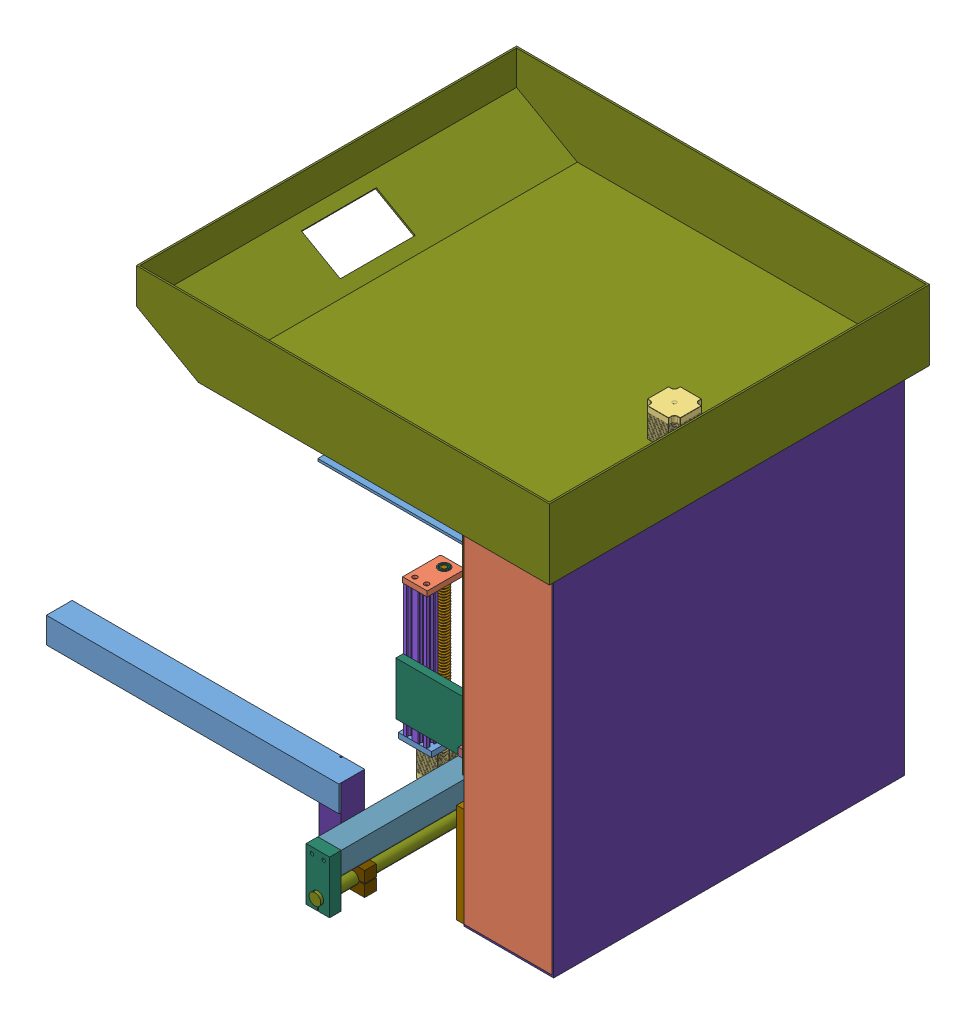
SolidWorks assembly Nueva Serigrafica, configuration Predeterminado. Lengths in mm.
Overall size (737.92 824.7 832.82).
71 component instances, 36 part files, 143 mates.
Components (placement in the parent):
- BASE DERECHA ACTUADOR LINEAL-1: BASE DERECHA ACTUADOR LINEAL [Predeterminado] at (30.0921 122.6863 -239.9315) x (0 1 0) z (0 0 -1) size (57 80 9)
- BASE LATERAL ACTUADOR LINEAL-1: BASE LATERAL ACTUADOR LINEAL [Predeterminado] at (22.5921 122.6863 182.0685) x (0 -1 0) z (0 0 1) size (42 65 9)
- SR Nema23 stepper motor with handwheel-1: SR Nema23 stepper motor with handwheel [Default] at (131.5379 118.3863 -326.6783) size (56.4 56.4 85)
- SOPORTE RODAMIENTO LATERAL-1: SOPORTE RODAMIENTO LATERAL [Predeterminado] at (32.5921 121.6863 -196.9315) x (0 1 0) z (0 0 -1) size (40 45 21)
- CARRO ACTUADOR LINEAL-1: CARRO ACTUADOR LINEAL [Predeterminado] at (40.0921 122.6863 164.8931) x (1 0 0) z (0 1 0) size (40 62 48)
- instrument ball bearing_68_am-1: instrument ball bearing_68_am [AFBMA 12.1.4.1 - 0080-19 - 10,DE,AC,10_68] at (40.0921 122.6863 188.0685) x (0 0 -1) z (1 0 0) size (6 19 19)
- instrument ball bearing_68_am-2: instrument ball bearing_68_am [AFBMA 12.1.4.1 - 0080-19 - 10,DE,AC,10_68] at (40.0921 122.6863 -199.9315) x (0 0 1) z (-1 0 0) size (6 19 19)
- VSlotRail_20X40X450-1: VSlotRail_20X40X450 [250mm] at (0.0921 132.6863 -239.9315) size (20 40 422)
- TORNILLO SINFINx400-1: TORNILLO SINFINx400 [Predeterminado] at (40.0921 122.6863 -77.9315) x (0 0 1) z (-1 0 0) size (289 16 16)
- SOPORTE ALUMINIO ACTUADOR SUPERIOR-1: SOPORTE ALUMINIO ACTUADOR SUPERIOR [Predeterminado] at (-22.6079 133.6863 -48.9315) x (0 0 -1) z (1 0 0) size (600 170 12.7)
- BARRA ACERO 20MM-1: BARRA ACERO 20MM [Predeterminado] at (30.0921 188.6863 -278.9315) x (0 0 1) z (-1 0 0) size (500 20 20)
- SOPORTE BARRA ACERO SUPERIOR-1: SOPORTE BARRA ACERO SUPERIOR [Predeterminado] at (30.0921 188.6863 206.3685) x (0 -1 0) z (0 0 1) size (40 55 12.7)
- SOPORTE BARRA ACERO SUPERIOR-2: SOPORTE BARRA ACERO SUPERIOR [Predeterminado] at (30.0921 188.6863 -281.2623) x (0 -1 0) z (0 0 1) size (40 55 12.7)
- CORREDERA SUPERIOR-1: CORREDERA SUPERIOR [Predeterminado] at (30.0921 188.6863 173.8931) x (0 -1 0) z (1 0 0) size (60 80 60)
- ANGULO 120X15X15X0.5In-1: ANGULO 120X15X15X0.5In [Predeterminado] at (72.7921 248.6863 133.8931) x (0 0 -1) z (0 1 0) size (120 150 150)
- RIEL SOPORTE-1: RIEL SOPORTE [Predeterminado] at (-57.2079 215.9863 133.8931) x (0 0 -1) z (-1 0 0) size (600 40 40)
- SOPORTE BARRA FRAME-1: SOPORTE BARRA FRAME [Predeterminado] at (-57.2079 190.9863 433.8931) x (-1 0 0) z (0 0 1) size (40 90 20)
- SOPORTE BARRA FRAME-2: SOPORTE BARRA FRAME [Predeterminado] at (-57.2079 190.9863 -186.1069) x (-1 0 0) z (0 0 1) size (40 90 20)
- BARRA ACERO 20MMX650-1: BARRA ACERO 20MMX650 [Predeterminado] at (-57.2079 165.9863 133.8931) x (1 0 0) z (0 1 0) size (20 650 20)
- RIEL 150mm-1: RIEL 150mm [Predeterminado] at (-97.2079 220.9863 373.8931) x (0 1 0) z (0 0 1) size (150 40 40)
- SOPORTE ACCESORIO-1: SOPORTE ACCESORIO [Predeterminado] at (-82.2079 165.9863 373.8931) x (0 -1 0) z (0 0 1) size (40 40 20)
- L ALUM 500X40X4mm-1: L ALUM 500X40X4mm [Predeterminado] at (-327.2079 291.9863 393.8931) x (0 -1 0) z (1 0 0) size (44 44 500)
- L ALUM 500X40X4mm-2: L ALUM 500X40X4mm [Predeterminado] at (-327.2079 291.9863 -106.1069) x (0 0 1) z (1 0 0) size (44 44 500)
- RIEL 150mm-2: RIEL 150mm [Predeterminado] at (-97.2079 220.9863 -86.1069) x (0 1 0) z (0 0 1) size (150 40 40)
- SOPORTE ACCESORIO-2: SOPORTE ACCESORIO [Predeterminado] at (-82.2079 165.9863 -106.1069) x (0 -1 0) z (0 0 1) size (40 40 20)
- SOPORTE LATERAL ALUMINIO SUPERIOR-1: SOPORTE LATERAL ALUMINIO SUPERIOR [Predeterminado] at (65.0921 348.6863 238.3685) x (0 -1 0) z (0 0 1) size (600 150 12.7)
- SOPORTE LATERAL ALUMINIO SUPERIOR-2: SOPORTE LATERAL ALUMINIO SUPERIOR [Predeterminado] at (65.0921 348.6863 -348.9315) x (0 -1 0) z (0 0 1) size (600 150 12.7)
- SOPORTE STEPPER DE REGISTRO-1: SOPORTE STEPPER DE REGISTRO [Predeterminado] at (-69.2332 426.7015 -48.9315) x (0 0 1) z (0.999998 -0.002087 0) size (60 80 12.7)
- SR Nema23 stepper motor with handwheel-2: SR Nema23 stepper motor with handwheel [Default] at (21.2027 421.3828 -140.9472) x (0 0 -1) z (-0.999998 0.002087 0) size (56.4 56.4 85)
- SOPORTE RODAMIENTO LATERAL-2: SOPORTE RODAMIENTO LATERAL [Predeterminado] at (-104.2383 424.2745 -47.9315) x (0 0 -1) z (-0.999998 0.002087 0) size (40 45 21)
- UNION STEPPER GUIA-1: UNION STEPPER GUIA [Predeterminado] at (-97.1914 446.7599 -48.9315) x (0 0 -1) z (0.999998 -0.002087 0) size (60 20 56)
- SOPORTE ACCESORIO-3: SOPORTE ACCESORIO [Predeterminado] at (-89.1601 461.7431 -18.9315) x (-0.999998 0.002087 0) z (0 0 -1) size (40 40 20)
- SOPORTE ACCESORIO-4: SOPORTE ACCESORIO [Predeterminado] at (-89.1601 461.7431 -58.9315) x (-0.999998 0.002087 0) z (0 0 -1) size (40 40 20)
- GUIA PARA STEPPER INFERIOR-1: GUIA PARA STEPPER INFERIOR [Predeterminado] at (-137.8182 481.8447 -48.9315) x (0 0 1) z (0.999998 -0.002087 0) size (30 70 12.7)
- GUIA CORREDERA INFERIOR-1: GUIA CORREDERA INFERIOR [Predeterminado] at (-255.0658 507.0895 -48.9315) x (-0.999998 0.002087 0) z (0 0 -1) size (275 20 90)
- instrument ball bearing_68_am-3: instrument ball bearing_68_am [AFBMA 12.1.4.1 - 0080-19 - 10,DE,AC,10_68] at (-110.254 416.7871 -48.9315) x (0.999998 -0.002087 0) z (0 0 1) size (6 19 19)
- SOPORTE EJE DE GIRO-1: SOPORTE EJE DE GIRO [Predeterminado] at (-89.1079 530.6739 -58.9315) x (0 0 1) z (1 0 0) size (20 120 30)
- ACTUADOR LINEAL PEQUENO-1: ACTUADOR LINEAL PEQUENO [Predeterminado] at (88.5921 626.8069 -58.72) x (-1 0 0) z (0 -1 0) size (80 57.27 308)
  - VSlotRail_20X40X225-1: VSlotRail_20X40X225 [250mm] at origin size (20 40 225)
  - BASE DERECHA ACTUADOR LINEAL-1: BASE DERECHA ACTUADOR LINEAL [Predeterminado] at (30 -10 0) x (0 1 0) z (0 0 -1) size (57 80 9)
  - BASE LATERAL ACTUADOR LINEAL-1: BASE LATERAL ACTUADOR LINEAL [Predeterminado] at (22.5 -10 225) x (0 -1 0) z (0 0 1) size (42 65 9)
  - SR Nema23 stepper motor with handwheel-1: SR Nema23 stepper motor with handwheel [Default] at (131.4458 -14.3001 -86.7468) size (56.4 56.4 85)
  - SOPORTE RODAMIENTO LATERAL-1: SOPORTE RODAMIENTO LATERAL [Predeterminado] at (32.5 -11 43) x (0 1 0) z (0 0 -1) size (40 45 21)
  - instrument ball bearing_68_am-1: instrument ball bearing_68_am [AFBMA 12.1.4.1 - 0080-19 - 10,DE,AC,10_68] at (40 -10 231) x (0 0 -1) z (1 0 0) size (6 19 19)
  - instrument ball bearing_68_am-2: instrument ball bearing_68_am [AFBMA 12.1.4.1 - 0080-19 - 10,DE,AC,10_68] at (40 -10 40) x (0 0 1) z (-1 0 0) size (6 19 19)
  - TORNILLO SINFIN-1: TORNILLO SINFIN [Predeterminado] at (40 -10 40) x (0 0 1) z (-1 0 0) size (214 16.03 16.03)
- placa soporte inferior 350x150-1: placa soporte inferior 350x150 [Predeterminado] at (111.2921 453.6863 -48.9315) x (0 0 1) z (-1 0 0) size (160 350 12.7)
- SOPORTE BARRA ACERO SUPERIOR-3: SOPORTE BARRA ACERO SUPERIOR [Predeterminado] at (58.5921 382.8069 11.0685) x (0 0 1) z (0 -1 0) size (40 55 12.7)
- SOPORTE BARRA ACERO SUPERIOR-4: SOPORTE BARRA ACERO SUPERIOR [Predeterminado] at (58.5921 612.8069 11.0685) x (0 0 1) z (0 -1 0) size (40 55 12.7)
- SOPORTE BARRA ACERO SUPERIOR-5: SOPORTE BARRA ACERO SUPERIOR [Predeterminado] at (58.5921 382.8069 -108.9315) x (0 0 1) z (0 -1 0) size (40 55 12.7)
- SOPORTE BARRA ACERO SUPERIOR-6: SOPORTE BARRA ACERO SUPERIOR [Predeterminado] at (58.5921 612.8069 -108.9315) x (0 0 1) z (0 -1 0) size (40 55 12.7)
- barra 20x250-1: barra 20x250 [Predeterminado] at (58.5921 365.8069 11.0685) size (20 250 20)
- barra 20x250-2: barra 20x250 [Predeterminado] at (58.5921 365.8069 -108.9315) x (0.999423 0 -0.033954) z (0.033954 0 0.999423) size (20 250 20)
- CORREDERA INFERIOR-1: CORREDERA INFERIOR [Predeterminado] at (58.5921 510.6627 -108.9315) x (0 0 1) z (-1 0 0) size (60 80 60)
- CORREDERA INFERIOR-2: CORREDERA INFERIOR [Predeterminado] at (58.5921 510.6627 11.0685) x (0 0 1) z (-1 0 0) size (60 80 60)
- SOPORTE EN T CORREDERAS INFERIORES-1: SOPORTE EN T CORREDERAS INFERIORES [Predeterminado] at (28.5921 510.6627 11.0685) x (0 0 1) z (-1 0 0) size (180 80.01 132.7)
- barra cuadrada espaciadora-1: barra cuadrada espaciadora [Predeterminado] at (105.0921 268.6863 -336.2315) x (1 0 0) z (0 -1 0) size (20 574.6 20)
- barra cuadrada espaciadora-2: barra cuadrada espaciadora [Predeterminado] at (105.0921 638.6863 -336.2315) x (1 0 0) z (0 -1 0) size (20 574.6 20)
- ANGULO 100X100X90XMEDIA-1: ANGULO 100X100X90XMEDIA [Predeterminado] at (-22.6079 48.6863 -7.4772) x (0 0 -1) z (0 1 0) size (112.7 350 90)
- ACTUADOR LINEAL PEQUENO-2: ACTUADOR LINEAL PEQUENO [Predeterminado] at (-362.6079 17.9863 -17.4772) x (0 0 -1) z (0 1 0) size (80 57.27 308)
  - VSlotRail_20X40X225-1: VSlotRail_20X40X225 [250mm] at origin size (20 40 225)
  - BASE DERECHA ACTUADOR LINEAL-1: BASE DERECHA ACTUADOR LINEAL [Predeterminado] at (30 -10 0) x (0 1 0) z (0 0 -1) size (57 80 9)
  - BASE LATERAL ACTUADOR LINEAL-1: BASE LATERAL ACTUADOR LINEAL [Predeterminado] at (22.5 -10 225) x (0 -1 0) z (0 0 1) size (42 65 9)
  - SR Nema23 stepper motor with handwheel-1: SR Nema23 stepper motor with handwheel [Default] at (131.4458 -14.3001 -86.7468) size (56.4 56.4 85)
  - SOPORTE RODAMIENTO LATERAL-1: SOPORTE RODAMIENTO LATERAL [Predeterminado] at (32.5 -11 43) x (0 1 0) z (0 0 -1) size (40 45 21)
  - instrument ball bearing_68_am-1: instrument ball bearing_68_am [AFBMA 12.1.4.1 - 0080-19 - 10,DE,AC,10_68] at (40 -10 231) x (0 0 -1) z (1 0 0) size (6 19 19)
  - instrument ball bearing_68_am-2: instrument ball bearing_68_am [AFBMA 12.1.4.1 - 0080-19 - 10,DE,AC,10_68] at (40 -10 40) x (0 0 1) z (-1 0 0) size (6 19 19)
  - TORNILLO SINFIN-1: TORNILLO SINFIN [Predeterminado] at (40 -10 40) x (0 0 1) z (-1 0 0) size (214 16.03 16.03)
- BASE SERIGRAFICA-1: BASE SERIGRAFICA [Predeterminado] at (160.7122 768.6863 -48.9315) x (-1 0 0) z (0 0 1) size (705.99 120 650)
- TAPA SUPERIOR-1: TAPA SUPERIOR [Predeterminado] at (140.0921 648.6863 -348.9315) x (-1 0 0) z (0 0 1) size (153 603 600)
- TAPA FRONTAL-1: TAPA FRONTAL [Predeterminado] at (-12.9079 458.6863 -48.9315) x (0 0 -1) z (1 0 0) size (600 380 3)
Mates (geometry in assembly coordinates):
- Concéntrica5: concentric aligned: cylinder of BASE DERECHA ACTUADOR LINEAL-1 through (63.0921 99.6863 -248.9315) axis (0 0 1) radius 2; cylinder of SR Nema23 stepper motor with handwheel-1 through (63.0921 99.6863 -253.9315) axis (0 0 1) radius 2.55
- Coincidente3: coincident anti-aligned: plane of BASE DERECHA ACTUADOR LINEAL-1 through (67.0921 97.1863 -248.9315) normal (0 0 -1); plane of SR Nema23 stepper motor with handwheel-1 through (39.5221 123.2563 -248.9315) normal (0 0 1)
- Paralelo2: parallel aligned: plane of BASE DERECHA ACTUADOR LINEAL-1 through (67.0921 94.1863 -248.9315) normal (0 -1 0); plane of SR Nema23 stepper motor with handwheel-1 through (39.5221 95.0563 -253.9315) normal (0 -1 0)
- Distancia1: distance = 34 mm anti-aligned: plane of SOPORTE RODAMIENTO LATERAL-1 through (52.0921 104.6863 -205.9315) normal (0 0 -1); plane of BASE DERECHA ACTUADOR LINEAL-1 through (67.0921 97.1863 -239.9315) normal (0 0 1)
- Coincidente5: coincident aligned: cylinder of BASE LATERAL ACTUADOR LINEAL-1 through (40.0921 122.6863 191.0685) axis (0 0 -1) radius 9.5; circle of SOPORTE RODAMIENTO LATERAL-1
- Concéntrica7: concentric anti-aligned: cylinder of BASE LATERAL ACTUADOR LINEAL-1 through (40.0921 122.6863 191.0685) axis (0 0 -1) radius 9.5; cylinder of CARRO ACTUADOR LINEAL-1 through (40.0921 122.6863 102.8931) axis (0 0 1) radius 8
- Concéntrica81: concentric aligned: cylinder of BASE LATERAL ACTUADOR LINEAL-1 through (40.0921 122.6863 191.0685) axis (0 0 -1) radius 9.5; cylinder of instrument ball bearing_68_am-1 through (40.0921 122.6863 208.706) axis (0 0 -1) radius 4
- Concéntrica91: concentric aligned: cylinder of SOPORTE RODAMIENTO LATERAL-1 through (40.0921 122.6863 -205.9315) axis (0 0 1) radius 9.5; cylinder of instrument ball bearing_68_am-2 through (40.0921 122.6863 -220.569) axis (0 0 1) radius 4
- Coincidente9: coincident aligned: plane of SOPORTE RODAMIENTO LATERAL-1 through (52.0921 104.6863 -196.9315) normal (0 0 1); plane of instrument ball bearing_68_am-2 through (40.0921 126.9863 -196.9315) normal (0 0 1)
- Coincidente10: coincident aligned: plane of BASE LATERAL ACTUADOR LINEAL-1 through (52.0921 140.6863 191.0685) normal (0 0 1); plane of instrument ball bearing_68_am-1 through (40.0921 128.3363 191.0685) normal (0 0 1)
- Concéntrica11: concentric anti-aligned: cylinder of BASE DERECHA ACTUADOR LINEAL-1 through (0.0921 132.6863 -248.9315) axis (0 0 1) radius 2; cylinder of VSlotRail_20X40X450-1 through (0.0921 132.6863 182.0685) axis (0 0 -1) radius 2.1
- Coincidente12: coincident anti-aligned: plane of BASE DERECHA ACTUADOR LINEAL-1 through (67.0921 97.1863 -239.9315) normal (0 0 1); plane of VSlotRail_20X40X450-1 through (0.0921 132.6863 -239.9315) normal (0 0 -1)
- Concéntrica12: concentric anti-aligned: cylinder of BASE LATERAL ACTUADOR LINEAL-1 through (0.0921 112.6863 186.5685) axis (0 0 1) radius 4; cylinder of VSlotRail_20X40X450-1 through (0.0921 112.6863 182.0685) axis (0 0 -1) radius 2.1
- Coincidente13: coincident anti-aligned: plane of BASE LATERAL ACTUADOR LINEAL-1 through (52.0921 140.6863 182.0685) normal (0 0 -1); plane of VSlotRail_20X40X450-1 through (0.0921 132.6863 182.0685) normal (0 0 1)
- Concéntrica13: concentric aligned: cylinder of instrument ball bearing_68_am-1 through (40.0921 122.6863 208.706) axis (0 0 -1) radius 4; cylinder of TORNILLO SINFINx400-1 through (40.0921 122.6863 191.0685) axis (0 0 -1) radius 4
- Coincidente14: coincident aligned: plane of BASE LATERAL ACTUADOR LINEAL-1 through (52.0921 140.6863 191.0685) normal (0 0 1); plane of TORNILLO SINFINx400-1 through (40.0921 122.6863 191.0685) normal (0 0 1)
- Coincidente15: coincident anti-aligned: plane of VSlotRail_20X40X450-1 through (-9.9079 128.0463 182.0685) normal (-1 0 0); plane of SOPORTE ALUMINIO ACTUADOR SUPERIOR-1 through (-9.9079 133.6863 -48.9315) normal (1 0 0)
- Paralelo3: parallel aligned: plane of SOPORTE RODAMIENTO LATERAL-1 through (55.0921 104.6863 -205.9315) normal (1 0 0); plane of VSlotRail_20X40X450-1 through (10.0921 108.0463 182.0685) normal (1 0 0)
- Coincidente17: coincident aligned: plane of BASE DERECHA ACTUADOR LINEAL-1 through (-9.9079 94.1863 -248.9315) normal (-1 0 0); plane of VSlotRail_20X40X450-1 through (-9.9079 128.0463 182.0685) normal (-1 0 0)
- Concéntrica92: concentric anti-aligned: cylinder of BASE LATERAL ACTUADOR LINEAL-1 through (0.0921 132.6863 186.5685) axis (0 0 1) radius 4; cylinder of VSlotRail_20X40X450-1 through (0.0921 132.6863 182.0685) axis (0 0 -1) radius 2.1
- Paralelo4: parallel aligned: plane of BASE DERECHA ACTUADOR LINEAL-1 through (70.0921 97.1863 -248.9315) normal (1 0 0); plane of CARRO ACTUADOR LINEAL-1 through (60.0921 146.6863 102.8931) normal (1 0 0)
- Coincidente19: coincident aligned: plane of SOPORTE BARRA ACERO SUPERIOR-1 through (30.0921 168.6863 219.0685) normal (0 -1 0); plane of SOPORTE BARRA ACERO SUPERIOR-2 through (30.0921 168.6863 -268.5623) normal (0 -1 0)
- Coincidente20: coincident aligned: plane of SOPORTE BARRA ACERO SUPERIOR-1 through (-9.9079 188.6863 219.0685) normal (-1 0 0); plane of SOPORTE BARRA ACERO SUPERIOR-2 through (-9.9079 188.6863 -268.5623) normal (-1 0 0)
- Coincidente21: coincident anti-aligned: plane of SOPORTE ALUMINIO ACTUADOR SUPERIOR-1 through (-9.9079 133.6863 -48.9315) normal (1 0 0); plane of SOPORTE BARRA ACERO SUPERIOR-1 through (-9.9079 188.6863 219.0685) normal (-1 0 0)
- Coincidente22: coincident anti-aligned: cylinder of BARRA ACERO 20MM-1 through (30.0921 188.6863 221.0685) axis (0 0 -1) radius 10; circle of SOPORTE BARRA ACERO SUPERIOR-1
- Ancho2: width aligned: plane of BARRA ACERO 20MM-1 through (30.0921 188.6863 -278.9315) normal (0 0 -1); plane of BARRA ACERO 20MM-1 through (30.0921 188.6863 221.0685) normal (0 0 1); plane of BASE DERECHA ACTUADOR LINEAL-1 through (67.0921 97.1863 -248.9315) normal (0 0 -1); plane of BASE LATERAL ACTUADOR LINEAL-1 through (52.0921 140.6863 191.0685) normal (0 0 1)
- Concéntrica93: concentric anti-aligned: cylinder of BARRA ACERO 20MM-1 through (30.0921 188.6863 221.0685) axis (0 0 -1) radius 10; cylinder of CORREDERA SUPERIOR-1 through (30.0921 188.6863 93.8931) axis (0 0 1) radius 10
- Paralelo5: parallel aligned: plane of SOPORTE ALUMINIO ACTUADOR SUPERIOR-1 through (-9.9079 133.6863 -48.9315) normal (1 0 0); plane of CORREDERA SUPERIOR-1 through (60.0921 158.6863 93.8931) normal (1 0 0)
- Ancho3: width aligned: plane of CARRO ACTUADOR LINEAL-1 through (40.0921 122.6863 102.8931) normal (0 0 -1); plane of CARRO ACTUADOR LINEAL-1 through (40.0921 122.6863 164.8931) normal (0 0 1); plane of CORREDERA SUPERIOR-1 through (30.0921 188.6863 93.8931) normal (0 0 -1); plane of CORREDERA SUPERIOR-1 through (30.0921 188.6863 173.8931) normal (0 0 1)
- Coincidente23: coincident aligned: plane of SOPORTE ALUMINIO ACTUADOR SUPERIOR-1 through (-9.9079 218.6863 251.0685) normal (0 1 0); plane of CORREDERA SUPERIOR-1 through (60.0921 218.6863 93.8931) normal (0 1 0)
- Distancia2: distance = 120 mm anti-aligned: plane of CORREDERA SUPERIOR-1 through (60.0921 218.6863 93.8931) normal (0 1 0); plane of CARRO ACTUADOR LINEAL-1 through (60.0921 98.6863 102.8931) normal (0 -1 0)
- Coincidente25: coincident anti-aligned: plane of CARRO ACTUADOR LINEAL-1 through (60.0921 146.6863 102.8931) normal (1 0 0); plane of ANGULO 120X15X15X0.5In-1 through (60.0921 225.9863 73.8931) normal (-1 0 0)
- Coincidente26: coincident aligned: plane of CARRO ACTUADOR LINEAL-1 through (60.0921 98.6863 102.8931) normal (0 -1 0); plane of ANGULO 120X15X15X0.5In-1 through (72.7921 98.6863 73.8931) normal (0 -1 0)
- Ancho4: width aligned: plane of ANGULO 120X15X15X0.5In-1 through (50.0921 225.9863 73.8931) normal (0 0 -1); plane of ANGULO 120X15X15X0.5In-1 through (50.0921 225.9863 193.8931) normal (0 0 1); plane of CARRO ACTUADOR LINEAL-1 through (40.0921 122.6863 102.8931) normal (0 0 -1); plane of CARRO ACTUADOR LINEAL-1 through (40.0921 122.6863 164.8931) normal (0 0 1)
- Distancia3: distance = 2 mm aligned: plane of SOPORTE BARRA ACERO SUPERIOR-1 through (30.0921 188.6863 219.0685) normal (0 0 1); plane of BARRA ACERO 20MM-1 through (30.0921 188.6863 221.0685) normal (0 0 1)
- Coincidente27: coincident anti-aligned: plane of ANGULO 120X15X15X0.5In-1 through (50.0921 235.9863 73.8931) normal (0 -1 0); plane of RIEL SOPORTE-1 through (-37.2079 235.9863 -166.1069) normal (0 1 0)
- Coincidente28: coincident aligned: plane of ANGULO 120X15X15X0.5In-1 through (-77.2079 248.6863 73.8931) normal (-1 0 0); plane of RIEL SOPORTE-1 through (-77.2079 235.9863 -166.1069) normal (-1 0 0)
- Ancho5: width aligned: plane of RIEL SOPORTE-1 through (-40.2079 198.9863 433.8931) normal (0 0 1); plane of RIEL SOPORTE-1 through (-40.2079 198.9863 -166.1069) normal (0 0 -1); plane of ANGULO 120X15X15X0.5In-1 through (50.0921 225.9863 193.8931) normal (0 0 1); plane of ANGULO 120X15X15X0.5In-1 through (50.0921 225.9863 73.8931) normal (0 0 -1)
- Concéntrica94: concentric anti-aligned: cylinder of RIEL SOPORTE-1 through (-67.2079 225.9863 423.8931) axis (0 0 1) radius 3; cylinder of SOPORTE BARRA FRAME-1 through (-67.2079 225.9863 453.8931) axis (0 0 -1) radius 3
- Concéntrica95: concentric anti-aligned: cylinder of RIEL SOPORTE-1 through (-47.2079 225.9863 423.8931) axis (0 0 1) radius 3; cylinder of SOPORTE BARRA FRAME-1 through (-47.2079 225.9863 453.8931) axis (0 0 -1) radius 3
- Coincidente29: coincident anti-aligned: plane of RIEL SOPORTE-1 through (-40.2079 198.9863 433.8931) normal (0 0 1); plane of SOPORTE BARRA FRAME-1 through (-57.2079 190.9863 433.8931) normal (0 0 -1)
- Concéntrica96: concentric aligned: cylinder of SOPORTE BARRA FRAME-1 through (-57.2079 165.9863 453.8931) axis (0 0 -1) radius 10; cylinder of SOPORTE BARRA FRAME-2 through (-57.2079 165.9863 -166.1069) axis (0 0 -1) radius 10
- Concéntrica97: concentric aligned: cylinder of SOPORTE BARRA FRAME-1 through (-47.2079 225.9863 453.8931) axis (0 0 -1) radius 3; cylinder of SOPORTE BARRA FRAME-2 through (-47.2079 225.9863 -166.1069) axis (0 0 -1) radius 3
- Coincidente30: coincident anti-aligned: plane of RIEL SOPORTE-1 through (-40.2079 198.9863 -166.1069) normal (0 0 -1); plane of SOPORTE BARRA FRAME-2 through (-57.2079 190.9863 -166.1069) normal (0 0 1)
- Concéntrica98: concentric anti-aligned: cylinder of SOPORTE BARRA FRAME-1 through (-57.2079 165.9863 453.8931) axis (0 0 -1) radius 10; cylinder of BARRA ACERO 20MMX650-1 through (-57.2079 165.9863 -191.1069) axis (0 0 1) radius 10
- Distancia4: distance = 5 mm aligned: plane of BARRA ACERO 20MMX650-1 through (-57.2079 165.9863 458.8931) normal (0 0 1); plane of SOPORTE BARRA FRAME-1 through (-57.2079 190.9863 453.8931) normal (0 0 1)
- Distancia5: distance = 100 mm aligned: plane of BASE DERECHA ACTUADOR LINEAL-1 through (67.0921 97.1863 -248.9315) normal (0 0 -1); plane of SOPORTE ALUMINIO ACTUADOR SUPERIOR-1 through (-9.9079 48.6863 -348.9315) normal (0 0 -1)
- Coincidente34: coincident anti-aligned: plane of RIEL SOPORTE-1 through (-77.2079 235.9863 -166.1069) normal (-1 0 0); plane of RIEL 150mm-1 through (-77.2079 295.9863 353.8931) normal (1 0 0)
- Paralelo7: parallel aligned: plane of SOPORTE BARRA FRAME-1 through (-57.2079 190.9863 453.8931) normal (0 0 1); plane of RIEL 150mm-1 through (-77.2079 295.9863 393.8931) normal (0 0 1)
- Coincidente35: coincident anti-aligned: plane of RIEL 150mm-1 through (-77.2079 295.9863 353.8931) normal (1 0 0); plane of SOPORTE ACCESORIO-1 through (-77.2079 185.9863 373.8931) normal (-1 0 0)
- Coincidente36: coincident aligned: plane of RIEL 150mm-1 through (-114.2079 145.9863 356.8931) normal (0 -1 0); plane of SOPORTE ACCESORIO-1 through (-82.2079 145.9863 393.8931) normal (0 -1 0)
- Concéntrica99: concentric anti-aligned: cylinder of BARRA ACERO 20MMX650-1 through (-57.2079 165.9863 -191.1069) axis (0 0 1) radius 10; cylinder of SOPORTE ACCESORIO-1 through (-57.2079 165.9863 393.8931) axis (0 0 -1) radius 10
- Coincidente37: coincident aligned: plane of RIEL 150mm-1 through (-77.2079 295.9863 393.8931) normal (0 0 1); plane of SOPORTE ACCESORIO-1 through (-82.2079 165.9863 393.8931) normal (0 0 1)
- Coincidente38: coincident anti-aligned: plane of L ALUM 500X40X4mm-1 through (-77.2079 289.9863 393.8931) normal (0 0 -1); plane of RIEL 150mm-1 through (-77.2079 295.9863 393.8931) normal (0 0 1)
- Coincidente39: coincident aligned: plane of RIEL 150mm-1 through (-114.2079 295.9863 356.8931) normal (0 1 0); plane of L ALUM 500X40X4mm-1 through (-77.2079 295.9863 397.8931) normal (0 1 0)
- Coincidente40: coincident aligned: plane of RIEL 150mm-1 through (-77.2079 295.9863 353.8931) normal (1 0 0); plane of L ALUM 500X40X4mm-1 through (-77.2079 289.9863 391.8931) normal (1 0 0)
- Coincidente42: coincident aligned: plane of L ALUM 500X40X4mm-2 through (-77.2079 289.9863 -104.1069) normal (1 0 0); plane of RIEL 150mm-2 through (-77.2079 295.9863 -106.1069) normal (1 0 0)
- Coincidente44: coincident aligned: plane of SOPORTE ACCESORIO-2 through (-82.2079 165.9863 -106.1069) normal (0 0 -1); plane of RIEL 150mm-2 through (-77.2079 295.9863 -106.1069) normal (0 0 -1)
- Coincidente45: coincident anti-aligned: plane of RIEL 150mm-2 through (-77.2079 295.9863 -106.1069) normal (1 0 0); plane of SOPORTE ACCESORIO-2 through (-77.2079 185.9863 -106.1069) normal (-1 0 0)
- Coincidente46: coincident aligned: plane of RIEL 150mm-2 through (-114.2079 145.9863 -103.1069) normal (0 -1 0); plane of SOPORTE ACCESORIO-2 through (-82.2079 145.9863 -86.1069) normal (0 -1 0)
- Concéntrica100: concentric anti-aligned: cylinder of BARRA ACERO 20MMX650-1 through (-57.2079 165.9863 -191.1069) axis (0 0 1) radius 10; cylinder of SOPORTE ACCESORIO-2 through (-57.2079 165.9863 -86.1069) axis (0 0 -1) radius 10
- Coincidente47: coincident anti-aligned: plane of L ALUM 500X40X4mm-2 through (-77.2079 289.9863 -106.1069) normal (0 0 1); plane of RIEL 150mm-2 through (-77.2079 295.9863 -106.1069) normal (0 0 -1)
- Coincidente48: coincident aligned: plane of L ALUM 500X40X4mm-1 through (-77.2079 291.9863 391.8931) normal (0 -1 0); plane of L ALUM 500X40X4mm-2 through (-77.2079 291.9863 -104.1069) normal (0 -1 0)
- Distancia6: distance = 60 mm aligned: plane of RIEL 150mm-1 through (-77.2079 295.9863 393.8931) normal (0 0 1); plane of SOPORTE BARRA FRAME-1 through (-57.2079 190.9863 453.8931) normal (0 0 1)
- Distancia7: distance = 500 mm anti-aligned: plane of L ALUM 500X40X4mm-2 through (-77.2079 289.9863 -106.1069) normal (0 0 1); plane of L ALUM 500X40X4mm-1 through (-77.2079 289.9863 393.8931) normal (0 0 -1)
- Coincidente51: coincident anti-aligned: plane of SOPORTE ALUMINIO ACTUADOR SUPERIOR-1 through (-9.9079 133.6863 -48.9315) normal (1 0 0); plane of SOPORTE LATERAL ALUMINIO SUPERIOR-1 through (-9.9079 648.6863 251.0685) normal (-1 0 0)
- Coincidente52: coincident aligned: plane of SOPORTE ALUMINIO ACTUADOR SUPERIOR-1 through (-9.9079 48.6863 251.0685) normal (0 0 1); plane of SOPORTE LATERAL ALUMINIO SUPERIOR-1 through (65.0921 348.6863 251.0685) normal (0 0 1)
- Coincidente53: coincident aligned: plane of SOPORTE ALUMINIO ACTUADOR SUPERIOR-1 through (-9.9079 48.6863 251.0685) normal (0 -1 0); plane of SOPORTE LATERAL ALUMINIO SUPERIOR-1 through (-9.9079 48.6863 251.0685) normal (0 -1 0)
- Coincidente54: coincident anti-aligned: plane of SOPORTE ALUMINIO ACTUADOR SUPERIOR-1 through (-9.9079 133.6863 -48.9315) normal (1 0 0); plane of SOPORTE LATERAL ALUMINIO SUPERIOR-2 through (-9.9079 648.6863 -336.2315) normal (-1 0 0)
- Coincidente55: coincident aligned: plane of SOPORTE ALUMINIO ACTUADOR SUPERIOR-1 through (-9.9079 48.6863 251.0685) normal (0 -1 0); plane of SOPORTE LATERAL ALUMINIO SUPERIOR-2 through (-9.9079 48.6863 -336.2315) normal (0 -1 0)
- Coincidente56: coincident aligned: plane of SOPORTE ALUMINIO ACTUADOR SUPERIOR-1 through (-9.9079 48.6863 -348.9315) normal (0 0 -1); plane of SOPORTE LATERAL ALUMINIO SUPERIOR-2 through (65.0921 348.6863 -348.9315) normal (0 0 -1)
- Concéntrica101: concentric aligned: cylinder of SOPORTE STEPPER DE REGISTRO-1 through (-56.5541 416.675 -48.9315) axis (-0.999998 0.002087 0) radius 7.5; cylinder of SR Nema23 stepper motor with handwheel-2 through (-46.5541 416.6541 -48.9315) axis (-0.999998 0.002087 0) radius 4
- Coincidente57: coincident anti-aligned: plane of SOPORTE STEPPER DE REGISTRO-1 through (-56.5332 426.675 -48.9315) normal (0.999998 -0.002087 0); plane of SR Nema23 stepper motor with handwheel-2 through (-56.5541 416.675 -48.9315) normal (-0.999998 0.002087 0)
- Paralelo8: parallel aligned: plane of SOPORTE STEPPER DE REGISTRO-1 through (-56.5332 426.675 -18.9315) normal (0 0 1); plane of SR Nema23 stepper motor with handwheel-2 through (-51.5541 416.6645 -20.7315) normal (0 0 1)
- Concéntrica102: concentric anti-aligned: cylinder of SR Nema23 stepper motor with handwheel-2 through (-46.5541 416.6541 -48.9315) axis (-0.999998 0.002087 0) radius 4; cylinder of SOPORTE RODAMIENTO LATERAL-2 through (-113.2539 416.7933 -48.9315) axis (0.999998 -0.002087 0) radius 9.5
- Paralelo9: parallel aligned: plane of SOPORTE STEPPER DE REGISTRO-1 through (-56.6167 386.675 -48.9315) normal (-0.002087 -0.999998 0); plane of SOPORTE RODAMIENTO LATERAL-2 through (-113.2853 401.7934 -30.9315) normal (-0.002087 -0.999998 0)
- Distancia8: distance = 35 mm anti-aligned: plane of SOPORTE STEPPER DE REGISTRO-1 through (-69.2332 426.7015 -48.9315) normal (-0.999998 0.002087 0); plane of SOPORTE RODAMIENTO LATERAL-2 through (-104.279 404.7746 -30.9315) normal (0.999998 -0.002087 0)
- Paralelo12: parallel aligned: plane of L ALUM 500X40X4mm-1 through (-77.2079 295.9863 397.8931) normal (0 0 1); plane of SOPORTE STEPPER DE REGISTRO-1 through (-56.5332 426.675 -18.9315) normal (0 0 1)
- Coincidente60: coincident anti-aligned: plane of SOPORTE STEPPER DE REGISTRO-1 through (-69.2332 426.7015 -48.9315) normal (-0.999998 0.002087 0); plane of UNION STEPPER GUIA-1 through (-69.1497 466.7014 -78.9315) normal (0.999998 -0.002087 0)
- Coincidente61: coincident anti-aligned: plane of SOPORTE RODAMIENTO LATERAL-2 through (-113.1913 446.7933 -27.9315) normal (0.002087 0.999998 0); plane of UNION STEPPER GUIA-1 through (-97.1914 446.7599 -48.9315) normal (-0.002087 -0.999998 0)
- Coincidente62: coincident aligned: plane of SOPORTE STEPPER DE REGISTRO-1 through (-56.5332 426.675 -78.9315) normal (0 0 -1); plane of UNION STEPPER GUIA-1 through (-69.1497 466.7014 -78.9315) normal (0 0 -1)
- Coincidente63: coincident anti-aligned: plane of UNION STEPPER GUIA-1 through (-97.1496 466.7598 -48.9315) normal (0.002087 0.999998 0); plane of SOPORTE ACCESORIO-3 through (-69.1497 466.7014 -18.9315) normal (-0.002087 -0.999998 0)
- Coincidente65: coincident anti-aligned: plane of UNION STEPPER GUIA-1 through (-97.1496 466.7598 -48.9315) normal (0.002087 0.999998 0); plane of SOPORTE ACCESORIO-4 through (-69.1497 466.7014 -58.9315) normal (-0.002087 -0.999998 0)
- Coincidente66: coincident aligned: plane of SOPORTE ACCESORIO-3 through (-109.16 461.7849 -38.9315) normal (-0.999998 0.002087 0); plane of SOPORTE ACCESORIO-4 through (-109.16 461.7849 -78.9315) normal (-0.999998 0.002087 0)
- Distancia10: distance = 20 mm anti-aligned: plane of SOPORTE ACCESORIO-3 through (-89.1601 461.7431 -38.9315) normal (0 0 -1); plane of SOPORTE ACCESORIO-4 through (-89.1601 461.7431 -58.9315) normal (0 0 1)
- Ancho6: width aligned: plane of SOPORTE ACCESORIO-3 through (-89.1601 461.7431 -18.9315) normal (0 0 1); plane of SOPORTE ACCESORIO-4 through (-89.1601 461.7431 -78.9315) normal (0 0 -1); plane of UNION STEPPER GUIA-1 through (-69.1497 466.7014 -18.9315) normal (0 0 1); plane of UNION STEPPER GUIA-1 through (-69.1497 466.7014 -78.9315) normal (0 0 -1)
- Coincidente67: coincident aligned: line of UNION STEPPER GUIA-1 through (-69.1497 466.7014 -18.9315) axis (0 0 -1); line of SOPORTE ACCESORIO-3 through (-69.1497 466.7014 -18.9315) axis (0 0 -1)
- Coincidente68: coincident anti-aligned: plane of UNION STEPPER GUIA-1 through (-125.1496 466.8183 -78.9315) normal (-0.999998 0.002087 0); plane of GUIA PARA STEPPER INFERIOR-1 through (-125.1183 481.8182 -48.9315) normal (0.999998 -0.002087 0)
- Coincidente69: coincident aligned: plane of UNION STEPPER GUIA-1 through (-97.1914 446.7599 -48.9315) normal (-0.002087 -0.999998 0); plane of GUIA PARA STEPPER INFERIOR-1 through (-125.1913 446.8183 -63.9315) normal (-0.002087 -0.999998 0)
- Ancho7: width aligned: plane of GUIA PARA STEPPER INFERIOR-1 through (-125.1913 446.8183 -33.9315) normal (0 0 1); plane of GUIA PARA STEPPER INFERIOR-1 through (-125.1913 446.8183 -63.9315) normal (0 0 -1); plane of UNION STEPPER GUIA-1 through (-69.1497 466.7014 -18.9315) normal (0 0 1); plane of UNION STEPPER GUIA-1 through (-69.1497 466.7014 -78.9315) normal (0 0 -1)
- Coincidente70: coincident anti-aligned: plane of GUIA PARA STEPPER INFERIOR-1 through (-125.1391 471.8182 -56.4315) normal (0 0 1); plane of GUIA CORREDERA INFERIOR-1 through (-255.0241 527.0894 -56.4315) normal (0 0 -1)
- Coincidente71: coincident aligned: plane of GUIA PARA STEPPER INFERIOR-1 through (-125.1183 481.8182 -48.9315) normal (0.999998 -0.002087 0); plane of GUIA CORREDERA INFERIOR-1 through (-125.0243 526.8181 -48.9315) normal (0.999998 -0.002087 0)
- Concéntrica1031: concentric aligned: cylinder of SOPORTE RODAMIENTO LATERAL-2 through (-113.2539 416.7933 -48.9315) axis (0.999998 -0.002087 0) radius 9.5; cylinder of instrument ball bearing_68_am-3 through (-130.8914 416.8301 -48.9315) axis (0.999998 -0.002087 0) radius 4
- Coincidente72: coincident: line of SOPORTE RODAMIENTO LATERAL-2 through (-113.2101 437.7933 -67.9315) axis (-0.002087 -0.999998 0); plane of instrument ball bearing_68_am-3 through (-113.2422 422.4433 -48.9315) normal (-0.999998 0.002087 0)
- Concéntrica104: concentric anti-aligned: cylinder of SOPORTE ACCESORIO-3 through (-89.1079 486.7431 -38.9315) axis (0 0 1) radius 10; cylinder of SOPORTE EJE DE GIRO-1 through (-89.1079 486.7431 -38.9315) axis (0 0 -1) radius 10
- Coincidente73: coincident anti-aligned: plane of SOPORTE ACCESORIO-3 through (-89.1601 461.7431 -38.9315) normal (0 0 -1); plane of SOPORTE EJE DE GIRO-1 through (-89.1079 530.6739 -38.9315) normal (0 0 1)
- Paralelo13: parallel aligned: plane of SOPORTE ALUMINIO ACTUADOR SUPERIOR-1 through (-22.6079 133.6863 -48.9315) normal (-1 0 0); plane of SOPORTE EJE DE GIRO-1 through (-104.1079 470.6739 -38.9315) normal (-1 0 0)
- Ancho8: width aligned: plane of SOPORTE EJE DE GIRO-1 through (-89.1079 530.6739 -38.9315) normal (0 0 1); plane of SOPORTE EJE DE GIRO-1 through (-89.1079 530.6739 -58.9315) normal (0 0 -1); plane of SOPORTE LATERAL ALUMINIO SUPERIOR-1 through (65.0921 348.6863 251.0685) normal (0 0 1); plane of SOPORTE LATERAL ALUMINIO SUPERIOR-2 through (65.0921 348.6863 -348.9315) normal (0 0 -1)
- Paralelo14: parallel aligned: plane of SOPORTE LATERAL ALUMINIO SUPERIOR-1 through (-9.9079 48.6863 251.0685) normal (0 -1 0); plane of ACTUADOR LINEAL PEQUENO-1/BASE LATERAL ACTUADOR LINEAL-1 through (36.5921 392.8069 -66.72) normal (0 -1 0)
- Paralelo15: parallel anti-aligned: plane of SOPORTE EJE DE GIRO-1 through (-74.1079 470.6739 -38.9315) normal (1 0 0); plane of ? through (28.5921 581.6627 -72.72) normal (-1 0 0)
- Ancho9: width anti-aligned: plane of placa soporte inferior 350x150-1 through (98.5921 278.6863 31.0685) normal (0 0 1); plane of placa soporte inferior 350x150-1 through (98.5921 278.6863 -128.9315) normal (0 0 -1); plane of SOPORTE LATERAL ALUMINIO SUPERIOR-2 through (65.0921 348.6863 -348.9315) normal (0 0 -1); plane of SOPORTE LATERAL ALUMINIO SUPERIOR-1 through (65.0921 348.6863 251.0685) normal (0 0 1)
- Coincidente76: coincident anti-aligned: plane of ACTUADOR LINEAL PEQUENO-1/VSlotRail_20X40X225-1 through (98.5921 401.8069 -54.0799) normal (1 0 0); plane of placa soporte inferior 350x150-1 through (98.5921 453.6863 -48.9315) normal (-1 0 0)
- Coincidente77: coincident anti-aligned: plane of placa soporte inferior 350x150-1 through (98.5921 453.6863 -48.9315) normal (-1 0 0); plane of SOPORTE BARRA ACERO SUPERIOR-3 through (98.5921 370.1069 11.0685) normal (1 0 0)
- Distancia11: distance = 10 mm anti-aligned: plane of SOPORTE BARRA ACERO SUPERIOR-3 through (58.5921 382.8069 11.0685) normal (0 1 0); plane of ACTUADOR LINEAL PEQUENO-1/BASE LATERAL ACTUADOR LINEAL-1 through (36.5921 392.8069 -66.72) normal (0 -1 0)
- Concéntrica105: concentric anti-aligned: cylinder of SOPORTE BARRA ACERO SUPERIOR-3 through (58.5921 370.1069 11.0685) axis (0 1 0) radius 10; cylinder of barra 20x250-1 through (58.5921 615.8069 11.0685) axis (0 -1 0) radius 10
- Concéntrica106: concentric anti-aligned: cylinder of SOPORTE BARRA ACERO SUPERIOR-6 through (58.5921 600.1069 -108.9315) axis (0 1 0) radius 10; cylinder of barra 20x250-2 through (58.5921 615.8069 -108.9315) axis (0 -1 0) radius 10
- Coincidente83: coincident aligned: plane of barra 20x250-1 through (58.5921 615.8069 11.0685) normal (0 1 0); plane of barra 20x250-2 through (58.5921 615.8069 -108.9315) normal (0 1 0)
- Distancia15: distance = 3 mm aligned: plane of barra 20x250-2 through (58.5921 615.8069 -108.9315) normal (0 1 0); plane of SOPORTE BARRA ACERO SUPERIOR-6 through (58.5921 612.8069 -108.9315) normal (0 1 0)
- Concéntrica107: concentric aligned: cylinder of barra 20x250-2 through (58.5921 615.8069 -108.9315) axis (0 -1 0) radius 10; cylinder of CORREDERA INFERIOR-1 through (58.5921 590.6627 -108.9315) axis (0 -1 0) radius 10
- Coincidente85: coincident aligned: plane of ? through (28.5921 581.6627 -72.72) normal (-1 0 0); plane of CORREDERA INFERIOR-1 through (28.5921 590.6627 -78.9315) normal (-1 0 0)
- Ancho10: width aligned: plane of CORREDERA INFERIOR-1 through (58.5921 590.6627 -108.9315) normal (0 1 0); plane of CORREDERA INFERIOR-1 through (58.5921 510.6627 -108.9315) normal (0 -1 0); plane of ? through (48.5921 581.6627 -48.72) normal (0 1 0); plane of ? through (48.5921 519.6627 -48.72) normal (0 -1 0)
- Concéntrica108: concentric aligned: cylinder of barra 20x250-1 through (58.5921 615.8069 11.0685) axis (0 -1 0) radius 10; cylinder of CORREDERA INFERIOR-2 through (58.5921 590.6627 11.0685) axis (0 -1 0) radius 10
- Paralelo18: parallel aligned: plane of CORREDERA INFERIOR-1 through (28.5921 590.6627 -78.9315) normal (-1 0 0); plane of CORREDERA INFERIOR-2 through (28.5921 590.6627 41.0685) normal (-1 0 0)
- Coincidente88: coincident aligned: plane of CORREDERA INFERIOR-1 through (58.5921 590.6627 -108.9315) normal (0 1 0); plane of CORREDERA INFERIOR-2 through (58.5921 590.6627 11.0685) normal (0 1 0)
- Ancho11: width aligned: plane of SOPORTE BARRA ACERO SUPERIOR-6 through (58.5921 600.1069 -128.9315) normal (0 0 -1); plane of SOPORTE BARRA ACERO SUPERIOR-4 through (58.5921 600.1069 31.0685) normal (0 0 1); plane of placa soporte inferior 350x150-1 through (98.5921 278.6863 -128.9315) normal (0 0 -1); plane of placa soporte inferior 350x150-1 through (98.5921 278.6863 31.0685) normal (0 0 1)
- EnPosición1: in place: plane of ? through (-76.2924 498.0536 41.0685) normal (-1 0 0); plane of ? through (-76.2924 0 0) normal (-1 0 0); moOrthogonalPlaneRef_w of ? through (-76.2924 498.0536 41.0685) normal (-1 0 0); line of ? through (-55 -76.2924 0) axis (0 0 1); plane of ? through (-76.2924 498.0536 41.0685) normal (-1 0 0); plane of ? through (-76.2924 0 0) normal (0 0 1); plane of CORREDERA INFERIOR-2 through (28.5921 590.6627 41.0685) normal (-1 0 0); unknown of SOPORTE EN T CORREDERAS INFERIORES-1
- Coincidente89: coincident aligned: plane of CORREDERA INFERIOR-2; plane of SOPORTE EN T CORREDERAS INFERIORES-1
- Coincidente90: coincident aligned: plane of CORREDERA INFERIOR-2 through (28.5921 510.6627 11.0685) normal (0 1 0); unknown of SOPORTE EN T CORREDERAS INFERIORES-1
- Coincidente91: coincident anti-aligned: plane of CORREDERA INFERIOR-2 through (28.5921 510.6627 11.0685) normal (0 0 -1); plane of SOPORTE EN T CORREDERAS INFERIORES-1 through (28.5921 510.6627 11.0685) normal (0 0 1)
- Distancia16: distance = 3.5 mm aligned: plane of barra cuadrada espaciadora-1 through (95.0921 278.6863 238.3685) normal (-1 0 0); plane of placa soporte inferior 350x150-1 through (98.5921 453.6863 -48.9315) normal (-1 0 0)
- Coincidente93: coincident anti-aligned: plane of placa soporte inferior 350x150-1 through (98.5921 278.6863 -128.9315) normal (0 -1 0); plane of barra cuadrada espaciadora-1 through (115.0921 278.6863 238.3685) normal (0 1 0)
- Coincidente94: coincident anti-aligned: plane of SOPORTE LATERAL ALUMINIO SUPERIOR-1 through (65.0921 348.6863 238.3685) normal (0 0 -1); plane of barra cuadrada espaciadora-1 through (105.0921 268.6863 238.3685) normal (0 0 1)
- Coincidente95: coincident aligned: plane of barra cuadrada espaciadora-1 through (95.0921 278.6863 238.3685) normal (-1 0 0); plane of barra cuadrada espaciadora-2 through (95.0921 648.6863 238.3685) normal (-1 0 0)
- Coincidente96: coincident anti-aligned: plane of placa soporte inferior 350x150-1 through (98.5921 628.6863 -128.9315) normal (0 1 0); plane of barra cuadrada espaciadora-2 through (115.0921 628.6863 238.3685) normal (0 -1 0)
- Coincidente97: coincident anti-aligned: plane of SOPORTE LATERAL ALUMINIO SUPERIOR-1 through (65.0921 348.6863 238.3685) normal (0 0 -1); plane of barra cuadrada espaciadora-2 through (105.0921 638.6863 238.3685) normal (0 0 1)
- Coincidente98: coincident aligned: plane of SOPORTE EJE DE GIRO-1 through (-74.1079 590.6739 -38.9315) normal (0 1 0); plane of SOPORTE EN T CORREDERAS INFERIORES-1 through (-104.1079 590.6739 -54.1315) normal (0 1 0)
- Distancia17: distance = 60 mm aligned: plane of GUIA PARA STEPPER INFERIOR-1 through (-125.1913 446.8183 -63.9315) normal (-0.002087 -0.999998 0); plane of GUIA CORREDERA INFERIOR-1 through (-255.0658 507.0895 -48.9315) normal (-0.002087 -0.999998 0)
- Coincidente99: coincident aligned: plane of SOPORTE LATERAL ALUMINIO SUPERIOR-1 through (-9.9079 648.6863 251.0685) normal (0 1 0); plane of barra cuadrada espaciadora-2 through (115.0921 648.6863 238.3685) normal (0 1 0)
- Coincidente100: coincident aligned: plane of SOPORTE EJE DE GIRO-1 through (-104.1079 470.6739 -38.9315) normal (-1 0 0); plane of SOPORTE EN T CORREDERAS INFERIORES-1 through (-104.1079 510.6627 11.0685) normal (-1 0 0)
- Coincidente101: coincident anti-aligned: plane of SOPORTE ALUMINIO ACTUADOR SUPERIOR-1 through (-22.6079 133.6863 -48.9315) normal (-1 0 0); plane of ANGULO 100X100X90XMEDIA-1 through (-22.6079 138.6863 -7.4772) normal (1 0 0)
- Coincidente102: coincident aligned: plane of SOPORTE ALUMINIO ACTUADOR SUPERIOR-1 through (-9.9079 48.6863 251.0685) normal (0 -1 0); plane of ANGULO 100X100X90XMEDIA-1 through (-36.6079 48.6863 -21.4772) normal (0 -1 0)
- Coincidente103: coincident anti-aligned: plane of ANGULO 100X100X90XMEDIA-1 through (-22.6079 48.6863 -7.4772) normal (0 0 -1); plane of ACTUADOR LINEAL PEQUENO-2/VSlotRail_20X40X225-1 through (-357.9679 242.9863 -7.4772) normal (0 0 1)
- Coincidente104: coincident aligned: plane of ANGULO 100X100X90XMEDIA-1 through (-372.6079 48.6863 5.2228) normal (-1 0 0); plane of ACTUADOR LINEAL PEQUENO-2/VSlotRail_20X40X225-1 through (-372.6079 242.9863 -12.8372) normal (-1 0 0)
- Distancia18: distance = 40 mm anti-aligned: plane of ACTUADOR LINEAL PEQUENO-2/BASE LATERAL ACTUADOR LINEAL-1 through (-370.6079 251.9863 -69.4772) normal (0 1 0); plane of L ALUM 500X40X4mm-1 through (-77.2079 291.9863 391.8931) normal (0 -1 0)
- Coincidente106: coincident anti-aligned: plane of SOPORTE LATERAL ALUMINIO SUPERIOR-1 through (-9.9079 648.6863 251.0685) normal (0 1 0); plane of BASE SERIGRAFICA-1 through (160.7122 648.6863 276.0685) normal (0 -1 0)
- Ancho12: width aligned: plane of BASE SERIGRAFICA-1 through (160.7122 768.6863 276.0685) normal (0 0 1); plane of BASE SERIGRAFICA-1 through (160.7122 768.6863 -373.9315) normal (0 0 -1); plane of SOPORTE LATERAL ALUMINIO SUPERIOR-1 through (65.0921 348.6863 251.0685) normal (0 0 1); plane of SOPORTE LATERAL ALUMINIO SUPERIOR-2 through (65.0921 348.6863 -348.9315) normal (0 0 -1)
- Coincidente107: coincident anti-aligned: plane of SOPORTE LATERAL ALUMINIO SUPERIOR-1 through (-9.9079 48.6863 251.0685) normal (0 -1 0); plane of TAPA SUPERIOR-1 through (140.0921 48.6863 251.0685) normal (0 1 0)
- Coincidente108: coincident aligned: plane of SOPORTE LATERAL ALUMINIO SUPERIOR-1 through (65.0921 348.6863 251.0685) normal (0 0 1); plane of TAPA SUPERIOR-1 through (140.0921 648.6863 251.0685) normal (0 0 1)
- Coincidente109: coincident anti-aligned: plane of SOPORTE LATERAL ALUMINIO SUPERIOR-1 through (140.0921 648.6863 251.0685) normal (1 0 0); plane of TAPA SUPERIOR-1 through (140.0921 648.6863 251.0685) normal (-1 0 0)
- Coincidente110: coincident anti-aligned: plane of SOPORTE LATERAL ALUMINIO SUPERIOR-1 through (-9.9079 648.6863 251.0685) normal (-1 0 0); plane of TAPA FRONTAL-1 through (-9.9079 458.6863 -48.9315) normal (1 0 0)
- Coincidente111: coincident anti-aligned: plane of BASE SERIGRAFICA-1 through (160.7122 648.6863 276.0685) normal (0 -1 0); plane of TAPA FRONTAL-1 through (-9.9079 648.6863 -348.9315) normal (0 1 0)
- Coincidente112: coincident aligned: plane of SOPORTE LATERAL ALUMINIO SUPERIOR-1 through (65.0921 348.6863 251.0685) normal (0 0 1); plane of TAPA FRONTAL-1 through (-9.9079 268.6863 251.0685) normal (0 0 1)
- Distancia19: distance = 25 mm anti-aligned: plane of barra cuadrada espaciadora-2 through (115.0921 648.6863 238.3685) normal (1 0 0); plane of TAPA SUPERIOR-1 through (140.0921 648.6863 251.0685) normal (-1 0 0)
